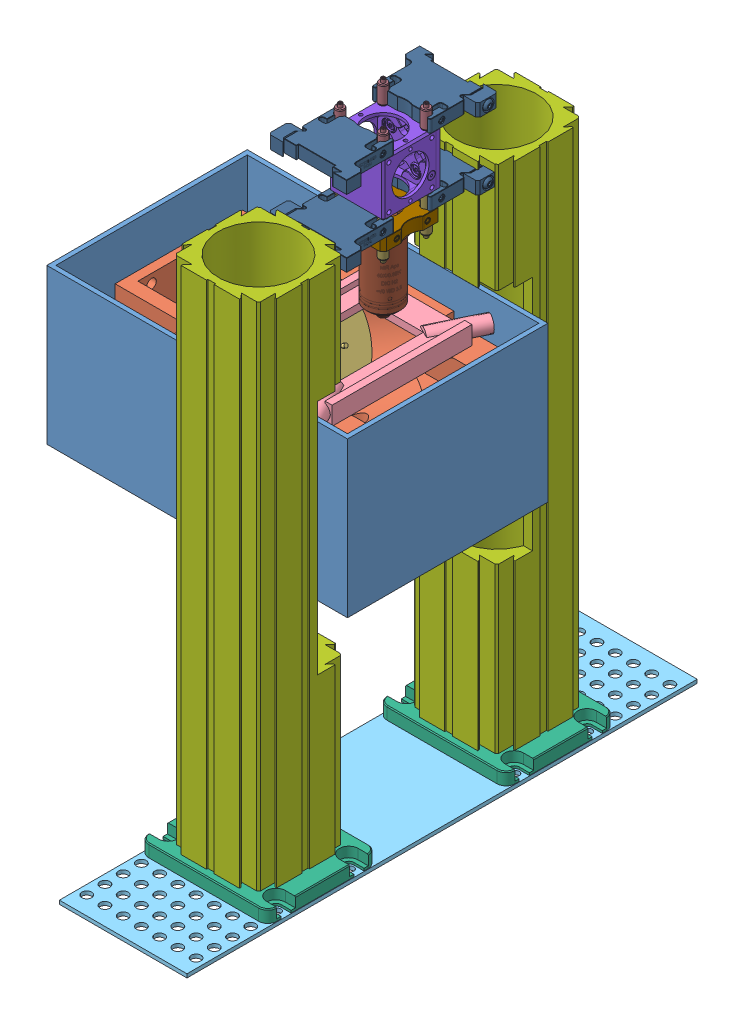
SolidWorks assembly DemoAssembly, configuration Default. Lengths in mm.
Overall size (209.55 415.14 355.6).
29 component instances, 15 part files, 16 mates.
Components (placement in the parent):
- Simple Framework-1: Simple Framework [Default] at origin size (209.55 107.95 139.7)
- 300 kHz Tank HP (5) Opticell-1: 300 kHz Tank HP (5) Opticell [Default] at (31.75 88.9 0) size (171.45 88.9 114.3)
- HP Tx-1: HP Tx [Default] at (-16.375 58.575 0) x (0.5 -0.866025 0) z (0 0 1) size (83.8 58.17 83.8)
- Opticell-1: Opticell [Default] at (36.6788 88.925 -0.195) size (76.36 12.75 129.72)
- Table SubAssembly-1: Table SubAssembly [Default] at (18.3002 -171.7184 0) x (0 0 -1) z (1 0 0) size (355.6 366.78 89.6)
  - Table-1: Table [Default] at origin size (355.6 2.54 88.9)
  - XT66P1-Solidworks-1: XT66P1-Solidworks [Default] at (-83.0224 2.286 37.592) x (-1 0 0) z (0 0 -1) size (76.2 8.89 89.28)
  - XT66P1-Solidworks-2: XT66P1-Solidworks [Default] at (83.0224 2.286 37.592) size (76.2 8.89 89.28)
  - KCB1-Solidworks-1: KCB1-Solidworks [Default] at (-24.13 99.7796 13.4747) x (0.000001 0 1) z (0 1 0) size (51.13 48.26 51.1) (hidden)
  - RCA1-Solidworks-1: RCA1-Solidworks [Default] at (-24.2926 205.6203 66.0649) x (0 0 -1) z (0 -1 0) size (56.5 73.55 8.89) (hidden)
  - RCA1-Solidworks-2: RCA1-Solidworks [Default] at (24.2926 108.2389 66.0649) x (0 0 -1) z (0 1 0) size (56.5 73.55 8.89) (hidden)
  - XT66-500-modified-1: XT66-500-modified [Default] at (-83.0224 511.176 37.592) x (0 0 -1) z (0 -1 0) size (66.02 67.06 355.6)
  - XT66-500-modified-2: XT66-500-modified [Default] at (83.0224 511.176 37.592) x (0 0 1) z (0 -1 0) size (66.02 67.06 355.6)
- Objective Sub-Assembly-1: Objective Sub-Assembly [Default] at (21.1998 -229.4603 -118.2913) x (0 0 1) z (0 -1 0) size (106.71 57.63 128.02)
  - CM1-DCH-Solidworks-1: CM1-DCH-Solidworks [Web Assembly] at (114.3818 -34.6924 -438.5894) x (0 -1 0) z (0 0 1) size (38.1 45.72 38.1)
  - CP16-Solidworks-1: CP16-Solidworks [Default] at (116.5677 -16.5858 -398.1348) x (0 -1 0) z (0 0 1) size (41.22 40.64 8.89)
  - RCA2-Solidworks-1: RCA2-Solidworks [Default] at (123.339 -21.2203 -499.1988) x (0 -1 0) z (0 0 1) size (56.73 41.06 8.89)
  - RCA2-Solidworks-2: RCA2-Solidworks [Default] at (105.4247 -48.1644 -499.1988) x (0 1 0) z (0 0 1) size (56.73 41.06 8.89)
  - N40X-NIR-Solidworks-1: N40X-NIR-Solidworks [Default] at (114.3819 -34.6923 -375.0894) x (0 0 1) z (0.875921 0.482454 0) size (61.98 27.94 27.94)
  - RCA2-Solidworks-3: RCA2-Solidworks [Default] at (105.4247 -48.1644 -452.2088) x (0 1 0) z (0 0 1) size (56.73 41.06 8.89)
  - RCA2-Solidworks-4: RCA2-Solidworks [Default] at (123.339 -21.2203 -452.2088) x (0 -1 0) z (0 0 1) size (56.73 41.06 8.89)
  - ER1-Solidworks-1: ER1-Solidworks [Default] at (100.293 -20.9473 -404.3535) x (-0.183947 -0.982936 0) z (0.982936 -0.183947 0) size (5.99 30.48 5.99)
  - ER1-Solidworks-2: ER1-Solidworks [Default] at (130.5299 -50.7349 -404.3535) x (0.020475 -0.99979 0) z (0.99979 0.020475 0) size (5.99 30.48 5.99)
  - ER1-Solidworks-3: ER1-Solidworks [Default] at (100.0093 -51.1105 -404.3535) x (-0.386185 -0.922421 0) z (0.922421 -0.386185 0) size (5.99 30.48 5.99)
  - ER1-Solidworks-4: ER1-Solidworks [Default] at (129.6817 -21.2139 -404.3535) x (-0.579753 -0.814792 0) z (0.814792 -0.579753 0) size (5.99 30.48 5.99)
  - ER05-Solidworks-1: ER05-Solidworks [Default] at (129.9725 -48.2584 -461.5035) x (0.933397 0.358845 0) z (-0.358845 0.933397 0) size (5.99 17.78 5.99)
  - ER05-Solidworks-2: ER05-Solidworks [Default] at (97.9162 -50.199 -461.5035) x (-0.886919 0.461926 0) z (-0.461926 -0.886919 0) size (5.99 17.78 5.99)
  - ER05-Solidworks-3: ER05-Solidworks [Default] at (128.9134 -21.1707 -461.5035) x (-0.900043 -0.4358 0) z (0.4358 -0.900043 0) size (5.99 17.78 5.99)
  - ER05-Solidworks-4: ER05-Solidworks [Default] at (100.2773 -18.4261 -461.5035) x (0.989892 0.141823 0) z (-0.141823 0.989892 0) size (5.99 17.78 5.99)
Mates (geometry in assembly coordinates):
- Coincident1: coordinate: point of Simple Framework-1; point of assembly
- Coincident2: coincident anti-aligned: plane of Simple Framework-1 through (0 0 0) normal (0 1 0); plane of 300 kHz Tank HP (5) Opticell-1 through (31.75 0 0) normal (0 -1 0)
- Concentric1: concentric aligned: cylinder of 300 kHz Tank HP (5) Opticell-1 through (-16.375 58.575 0) axis (-0.866025 -0.5 0) radius 42.545; cylinder of HP Tx-1 through (-16.375 58.575 0) axis (-0.866025 -0.5 0) radius 41.9
- Coincident3: coincident anti-aligned: plane of 300 kHz Tank HP (5) Opticell-1 through (-18.3925 62.0694 0) normal (0.866025 0.5 0); plane of HP Tx-1 through (-16.375 58.575 0) normal (-0.866025 -0.5 0)
- Coincident8: coincident anti-aligned: plane of 300 kHz Tank HP (5) Opticell-1 through (31.75 82.55 0) normal (0 1 0); plane of Opticell-1 through (36.6788 82.55 -0.195) normal (0 -1 0)
- Parallel2: parallel aligned: plane of 300 kHz Tank HP (5) Opticell-1 through (88.9 0 50.8) normal (1 0 0); plane of Opticell-1 through (72.7338 91.425 48.505) normal (1 0 0)
- Coincident9: coincident anti-aligned: plane of 300 kHz Tank HP (5) Opticell-1 through (0.6238 82.55 -48.895) normal (1 0 0); plane of Opticell-1 through (0.6238 91.425 48.505) normal (-1 0 0)
- Coincident14: coincident anti-aligned: plane of 300 kHz Tank HP (5) Opticell-1 through (0.6238 82.55 -48.895) normal (0 0 1); plane of Opticell-1 through (0.6238 91.425 -48.895) normal (0 0 -1)
- Concentric2: concentric aligned: circle of Simple Framework-1; circle of 300 kHz Tank HP (5) Opticell-1
- Concentric3: concentric aligned: circle of Simple Framework-1; circle of 300 kHz Tank HP (5) Opticell-1
- Coincident15: coincident anti-aligned: plane of Table SubAssembly-1/Table-1 through (18.3002 -171.7184 0) normal (0 0 -1); plane of assembly through (0 0 0) normal (0 0 1)
- Parallel3: parallel aligned: plane of 300 kHz Tank HP (5) Opticell-1 through (88.9 0 50.8) normal (1 0 0); plane of Table SubAssembly-1/XT66-500-modified-2 through (88.9 -160.5424 -103.3604) normal (1 0 0)
- Coincident16: coincident aligned: plane of 300 kHz Tank HP (5) Opticell-1 through (88.9 0 50.8) normal (1 0 0); plane of Table SubAssembly-1/XT66-500-modified-2 through (88.9 -160.5424 -103.3604) normal (1 0 0)
- Coincident17: coincident anti-aligned: plane of Table SubAssembly-1/XT66-500-modified-2 through (38.6207 -160.5424 -53.9094) normal (0 0 1); plane of Objective Sub-Assembly-1/RCA2-Solidworks-3 through (41.0466 181.1891 -53.9094) normal (0 0 -1)
- Parallel4: parallel aligned: plane of Table SubAssembly-1/XT66-500-modified-2 through (22.8844 -160.5424 -62.6845) normal (-1 0 0); plane of Objective Sub-Assembly-1/RCA2-Solidworks-3 through (35.5722 181.1891 -17.4857) normal (-1 0 0)
- Coincident19: coincident anti-aligned: plane of Table SubAssembly-1/Table-1 through (55.8922 -171.7184 0) normal (1 0 0); plane of Objective Sub-Assembly-1 through (55.8922 -229.4603 -118.2913) normal (-1 0 0)
